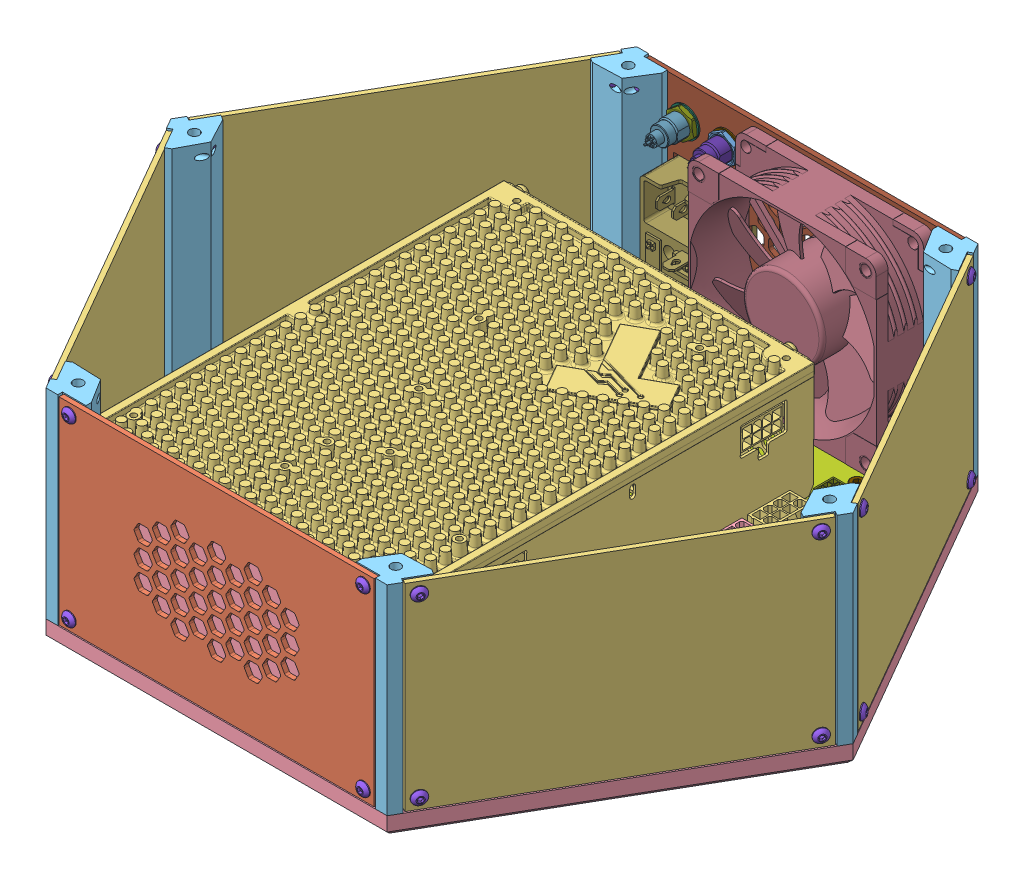
SolidWorks assembly base_assembly, configuration Default. Lengths in mm.
Overall size (362.5 93.4 376.72).
538 component instances, 72 part files, 51 mates.
Components (placement in the parent):
- psu_assembly-1: psu_assembly [Default] at (-81.5 8 97.5737) x (0 0 1) z (-1 0 0) size (187.35 61.91 139.14)
  - psu_mount-1: psu_mount [Default] at (-68 0 0) x (0 0 -1) z (1 0 0) size (39 54 68)
  - socket head cap screw_am-1: socket head cap screw_am [B18.3.1M - 3 x 0.5 x 8 Hex SHCS -- 8NHX] at (-64.25 14 3) x (0 0 -1) z (-0.998649 -0.051963 0) size (11 5.5 5.5)
  - socket head cap screw_am-2: socket head cap screw_am [B18.3.1M - 3 x 0.5 x 8 Hex SHCS -- 8NHX] at (-3.75 14 3) x (0 0 -1) z (-0.999942 -0.010799 0) size (11 5.5 5.5)
  - socket head cap screw_am-3: socket head cap screw_am [B18.3.1M - 3 x 0.5 x 8 Hex SHCS -- 8NHX] at (-3.75 50 3) x (0 0 -1) z (-0.998649 -0.051963 0) size (11 5.5 5.5)
  - IPC-5-1: IPC-5 [Default] at (-43.0401 19.0478 -84.9759) x (1 0 0) z (0 0.008727 0.999962) size (187.35 57.37 132.1)
- frame_bottom_assembly-1: frame_bottom_assembly [Default] at origin size (362.5 93.4 376.72)
  - bottom_plate_detail-1: bottom_plate_detail [Default] at (0 8 0) x (-0.5 0 -0.866025) z (-0.866025 0 0.5) size (290 8 251.15)
  - frame_pillar-1: frame_pillar [Default] at (72.5 8 -125.5737) x (-1 0 0) z (0 0 -1) size (20.77 85 15.16)
  - frame_pillar-3: frame_pillar [Default] at (-72.5 8 -125.5737) x (-0.5 0 0.866025) z (-0.866025 0 -0.5) size (20.77 85 15.16)
  - frame_pillar-4: frame_pillar [Default] at (-145 8 0) x (0.5 0 0.866025) z (-0.866025 0 0.5) size (20.77 85 15.16)
  - frame_pillar-5: frame_pillar [Default] at (-72.5 8 125.5737) size (20.77 85 15.16)
  - frame_pillar-6: frame_pillar [Default] at (72.5 8 125.5737) x (0.5 0 -0.866025) z (0.866025 0 0.5) size (20.77 85 15.16)
  - frame_pillar-7: frame_pillar [Default] at (145 8 0) x (-0.5 0 -0.866025) z (0.866025 0 -0.5) size (20.77 85 15.16)
  - socket countersunk head screw_am-5: socket countersunk head screw_am [B18.3.5M - 5 x 0.8 x 12 Socket FCHS  -- 12N] at (-70 0 38.5737) x (0 1 0) z (0 0 1) size (12 9.75 9.75)
  - socket countersunk head screw_am-6: socket countersunk head screw_am [B18.3.5M - 5 x 0.8 x 12 Socket FCHS  -- 12N] at (-50 0 38.5737) x (0 1 0) z (-0.110565 0 -0.993869) size (12 9.75 9.75)
  - socket countersunk head screw_am-7: socket countersunk head screw_am [B18.3.5M - 5 x 0.8 x 12 Socket FCHS  -- 12N] at (-50 0 88.5737) x (0 1 0) z (0 0 1) size (12 9.75 9.75)
  - socket countersunk head screw_am-8: socket countersunk head screw_am [B18.3.5M - 5 x 0.8 x 12 Socket FCHS  -- 12N] at (-70 0 88.5737) x (0 1 0) z (0 0 1) size (12 9.75 9.75)
  - socket countersunk head screw_am-9: socket countersunk head screw_am [B18.3.5M - 5 x 0.8 x 16 Socket FCHS  -- 16N] at (67.5 -0.4 116.9134) x (0 1 0) z (0 0 1) size (16 9.75 9.75)
  - socket countersunk head screw_am-10: socket countersunk head screw_am [B18.3.5M - 5 x 0.8 x 16 Socket FCHS  -- 16N] at (-67.5 -0.4 116.9134) x (0 1 0) z (0 0 1) size (16 9.75 9.75)
  - socket countersunk head screw_am-11: socket countersunk head screw_am [B18.3.5M - 5 x 0.8 x 16 Socket FCHS  -- 16N] at (-135 -0.4 0) x (0 1 0) z (0 0 1) size (16 9.75 9.75)
  - socket countersunk head screw_am-12: socket countersunk head screw_am [B18.3.5M - 5 x 0.8 x 16 Socket FCHS  -- 16N] at (-67.5 -0.4 -116.9134) x (0 1 0) z (0 0 1) size (16 9.75 9.75)
  - socket countersunk head screw_am-13: socket countersunk head screw_am [B18.3.5M - 5 x 0.8 x 16 Socket FCHS  -- 16N] at (67.5 -0.4 -116.9134) x (0 1 0) z (0 0 1) size (16 9.75 9.75)
  - socket countersunk head screw_am-14: socket countersunk head screw_am [B18.3.5M - 5 x 0.8 x 16 Socket FCHS  -- 16N] at (135 -0.4 0) x (0 1 0) z (0 0 1) size (16 9.75 9.75)
  - bottom_plate_cover-1: bottom_plate_cover [Default] at (124.7077 7 -108) x (-1 0 0) z (0 0 -1) size (247.87 1 216)
  - socket button head cap screw_am-1: socket button head cap screw_am [B18.3.4M - 3 x 0.5 x 6 SBHCS --N] at (120 9.65 0) x (0 -1 0) z (0 0 1) size (7.65 5.7 5.7) (hidden)
  - socket button head cap screw_am-2: socket button head cap screw_am [B18.3.4M - 3 x 0.5 x 6 SBHCS --N] at (60 9.65 103.923) x (0 -1 0) z (0 0 1) size (7.65 5.7 5.7) (hidden)
  - socket button head cap screw_am-3: socket button head cap screw_am [B18.3.4M - 3 x 0.5 x 6 SBHCS --N] at (-120 9.65 0) x (0 -1 0) z (0 0 1) size (7.65 5.7 5.7)
  - socket button head cap screw_am-4: socket button head cap screw_am [B18.3.4M - 3 x 0.5 x 6 SBHCS --N] at (-60 9.65 -103.923) x (0 -1 0) z (0 0 1) size (7.65 5.7 5.7)
  - socket button head cap screw_am-5: socket button head cap screw_am [B18.3.4M - 3 x 0.5 x 6 SBHCS --N] at (60 9.65 -103.923) x (0 -1 0) z (0 0 1) size (7.65 5.7 5.7)
  - nutsert_M3-4: nutsert_M3 [Default] at (60 5.5 -86.077) x (0.927804 0 -0.373067) z (0.373067 0 0.927804) size (5.3 2.75 5.3)
  - M3_standoff-1: M3_standoff [Default] at (60 8 -86.077) size (6.35 11 5.5)
  - M3_standoff-2: M3_standoff [Default] at (120 8 0) x (0.382257 0 -0.924056) z (0.924056 0 0.382257) size (6.35 11 5.5)
  - M3_standoff-3: M3_standoff [Default] at (60 8 103.923) size (6.35 11 5.5)
  - nutsert_M3-5: nutsert_M3 [Default] at (-90 5.5 -6.43) x (0.927804 0 -0.373067) z (0.373067 0 0.927804) size (5.3 2.75 5.3)
  - nutsert_M3-6: nutsert_M3 [Default] at (-110 5.5 13.57) x (0.927804 0 -0.373067) z (0.373067 0 0.927804) size (5.3 2.75 5.3)
  - nutsert_M3-7: nutsert_M3 [Default] at (-90 5.5 13.57) x (0.927804 0 -0.373067) z (0.373067 0 0.927804) size (5.3 2.75 5.3)
  - nutsert_M3-8: nutsert_M3 [Default] at (-90 5.5 33.57) x (0.927804 0 -0.373067) z (0.373067 0 0.927804) size (5.3 2.75 5.3)
  - nutsert_M3-9: nutsert_M3 [Default] at (-90 5.5 -26.43) x (0.927804 0 -0.373067) z (0.373067 0 0.927804) size (5.3 2.75 5.3)
- electronics_panel-1: electronics_panel [Default] at (-22.8265 182.5758 -40.206) x (-1 0 0) z (0 -1 0) size (134 36.39 84)
  - side_cover_fan-1: side_cover_fan [Default] at (-89.8265 83.3677 174.0758) size (134 2 84)
  - IEC 320 Switched-1: IEC 320 Switched [Default] at (4.4235 85.3677 118.9258) x (0 0 1) z (-1 0 0) size (58.1 34.87 32.67)
  - Noctua nf-a8-pwm fan 80x80x25-1: Noctua nf-a8-pwm fan 80x80x25 [По умолчанию] at (-39.0776 83.4677 131.8269) x (1 0 0.00003) z (0 -1 0) size (80 80 27.24)
  - socket button head cap screw_am-1: socket button head cap screw_am [B18.3.4M - 4 x 0.7 x 4 SBHCS --N] at (-74.5765 87.5677 96.3258) x (0 -1 0) z (0 0 1) size (6.2 7.6 7.6)
  - socket button head cap screw_am-2: socket button head cap screw_am [B18.3.4M - 4 x 0.7 x 4 SBHCS --N] at (-3.0765 87.5677 96.3258) x (0 -1 0) z (0 0 1) size (6.2 7.6 7.6)
  - socket button head cap screw_am-3: socket button head cap screw_am [B18.3.4M - 4 x 0.7 x 4 SBHCS --N] at (-3.0765 87.5677 167.8258) x (0 -1 0) z (0 0 1) size (6.2 7.6 7.6)
  - socket button head cap screw_am-4: socket button head cap screw_am [B18.3.4M - 4 x 0.7 x 4 SBHCS --N] at (-74.5765 87.5677 167.8258) x (0 -1 0) z (0 0 1) size (6.2 7.6 7.6)
  - egg_0b_307_cll-1: egg_0b_307_cll [Default] at (26.9235 88.8686 104.5758) x (-1 0 0) z (0 -1 0) size (12.77 13.42 20.7)
    - egg_0b_307_cll_1-1: egg_0b_307_cll_1 [Default] at (0 0 2.3009) size (10 10 20.7)
    - egg_0b_307_cll_2-1: egg_0b_307_cll_2 [Default] at (0 0 -1.0491) size (12.5 12.5 1.36)
    - egg_0b_307_cll_3-1: egg_0b_307_cll_3 [Default] at (0 0 -1.2991) size (12.77 13.42 2.93)
  - egg_0b_309_cll-1: egg_0b_309_cll [Default] at (8.9235 86.5677 104.5758) x (1 0 0) z (0 -1 0) size (12.5 12.5 20.23)
    - egg_0b_309_cll_1-1: egg_0b_309_cll_1 [Default] at origin size (10 10 20.23)
    - egg_0b_309_cll_2-1: egg_0b_309_cll_2 [Default] at (0 0 -4.6) size (12.5 12.5 1.3)
    - egg_0b_309_cll_3-1: egg_0b_309_cll_3 [Default] at (0 0 -4.85) size (11 12.4 2.02)
- socket button head cap screw_am-2: socket button head cap screw_am [B18.3.4M - 3 x 0.5 x 10 SBHCS --N] at (78.9289 13 -117.7384) x (-0.866025 0 0.5) z (-0.480675 0.27533 -0.832553) size (11.65 5.7 5.7)
- socket button head cap screw_am-3: socket button head cap screw_am [B18.3.4M - 3 x 0.5 x 10 SBHCS --N] at (141.4289 13 -9.4853) x (-0.866025 0 0.5) z (-0.480675 0.27533 -0.832553) size (11.65 5.7 5.7)
- socket button head cap screw_am-4: socket button head cap screw_am [B18.3.4M - 3 x 0.5 x 10 SBHCS --N] at (141.4289 88 -9.4853) x (-0.866025 0 0.5) z (-0.20533 0.911789 -0.355642) size (11.65 5.7 5.7)
- socket button head cap screw_am-5: socket button head cap screw_am [B18.3.4M - 3 x 0.5 x 10 SBHCS --N] at (78.9289 88 -117.7384) x (-0.866025 0 0.5) z (-0.480675 0.27533 -0.832553) size (11.65 5.7 5.7)
- socket button head cap screw_am-23: socket button head cap screw_am [B18.3.4M - 3 x 0.5 x 10 SBHCS --N] at (62.5 88 -127.2237) x (0 0 1) z (-0.900742 0.434355 0) size (11.65 5.7 5.7)
- socket button head cap screw_am-24: socket button head cap screw_am [B18.3.4M - 3 x 0.5 x 10 SBHCS --N] at (-62.5 88 -127.2237) x (0 0 1) z (-0.900742 0.434355 0) size (11.65 5.7 5.7)
- socket button head cap screw_am-25: socket button head cap screw_am [B18.3.4M - 3 x 0.5 x 10 SBHCS --N] at (-62.5 13 -127.2237) x (0 0 1) z (-0.900742 0.434355 0) size (11.65 5.7 5.7)
- socket button head cap screw_am-26: socket button head cap screw_am [B18.3.4M - 3 x 0.5 x 10 SBHCS --N] at (62.5 13 -127.2237) x (0 0 1) z (-0.900742 0.434355 0) size (11.65 5.7 5.7)
- side_cover_vent-1: side_cover_vent [Default] at (-67 8.5 123.5737) x (1 0 0) z (0 -1 0) size (134 2 84)
- side_cover_full-1: side_cover_full [Default] at (73.5179 92.5 -119.8105) x (0.5 0 0.866025) z (0 1 0) size (134 2 84)
- socket button head cap screw_am-27: socket button head cap screw_am [B18.3.4M - 3 x 0.5 x 10 SBHCS --N] at (-62.5 88 127.2237) x (0 0 -1) z (0.743296 -0.668962 0) size (11.65 5.7 5.7)
- socket button head cap screw_am-28: socket button head cap screw_am [B18.3.4M - 3 x 0.5 x 10 SBHCS --N] at (62.5 88 127.2237) x (0 0 -1) z (0.743296 -0.668962 0) size (11.65 5.7 5.7)
- socket button head cap screw_am-29: socket button head cap screw_am [B18.3.4M - 3 x 0.5 x 10 SBHCS --N] at (62.5 13 127.2237) x (0 0 -1) z (0.743296 -0.668962 0) size (11.65 5.7 5.7)
- socket button head cap screw_am-30: socket button head cap screw_am [B18.3.4M - 3 x 0.5 x 10 SBHCS --N] at (-62.5 13 127.2237) x (0 0 -1) z (0.743296 -0.668962 0) size (11.65 5.7 5.7)
- demci_filter_0887-1: demci_filter_0887 [Default] at (0 50.5 122.3737) x (1 0 0) z (0 -1 0) size (97 2.4 71)
- socket button head cap screw_am-31: socket button head cap screw_am [B18.3.4M - 3 x 0.5 x 10 SBHCS --N] at (-78.9289 13 -117.7384) x (0.866025 0 0.5) z (-0.480675 0.27533 0.832553) size (11.65 5.7 5.7)
- socket button head cap screw_am-32: socket button head cap screw_am [B18.3.4M - 3 x 0.5 x 10 SBHCS --N] at (-141.4289 13 9.4853) x (0.866025 0 -0.5) z (0.480675 0.27533 0.832553) size (11.65 5.7 5.7)
- socket button head cap screw_am-33: socket button head cap screw_am [B18.3.4M - 3 x 0.5 x 10 SBHCS --N] at (78.9289 13 117.7384) x (-0.866025 0 -0.5) z (0.480675 0.27533 -0.832553) size (11.65 5.7 5.7)
- socket button head cap screw_am-34: socket button head cap screw_am [B18.3.4M - 3 x 0.5 x 10 SBHCS --N] at (-141.4289 13 -9.4853) x (0.866025 0 0.5) z (-0.480675 0.27533 0.832553) size (11.65 5.7 5.7)
- socket button head cap screw_am-35: socket button head cap screw_am [B18.3.4M - 3 x 0.5 x 10 SBHCS --N] at (-78.9289 13 117.7384) x (0.866025 0 -0.5) z (0.480675 0.27533 0.832553) size (11.65 5.7 5.7)
- socket button head cap screw_am-36: socket button head cap screw_am [B18.3.4M - 3 x 0.5 x 10 SBHCS --N] at (141.4289 13 9.4853) x (-0.866025 0 -0.5) z (0.480675 0.27533 -0.832553) size (11.65 5.7 5.7)
- socket button head cap screw_am-37: socket button head cap screw_am [B18.3.4M - 3 x 0.5 x 10 SBHCS --N] at (-141.4289 88 -9.4853) x (0.866025 0 0.5) z (-0.480675 0.27533 0.832553) size (11.65 5.7 5.7)
- socket button head cap screw_am-38: socket button head cap screw_am [B18.3.4M - 3 x 0.5 x 10 SBHCS --N] at (-78.9289 88 117.7384) x (0.866025 0 -0.5) z (0.480675 0.27533 0.832553) size (11.65 5.7 5.7)
- socket button head cap screw_am-39: socket button head cap screw_am [B18.3.4M - 3 x 0.5 x 10 SBHCS --N] at (141.4289 88 9.4853) x (-0.866025 0 -0.5) z (0.480675 0.27533 -0.832553) size (11.65 5.7 5.7)
- socket button head cap screw_am-40: socket button head cap screw_am [B18.3.4M - 3 x 0.5 x 10 SBHCS --N] at (-78.9289 88 -117.7384) x (0.866025 0 0.5) z (-0.20533 0.911789 0.355642) size (11.65 5.7 5.7)
- socket button head cap screw_am-41: socket button head cap screw_am [B18.3.4M - 3 x 0.5 x 10 SBHCS --N] at (-141.4289 88 9.4853) x (0.866025 0 -0.5) z (0.20533 0.911789 0.355642) size (11.65 5.7 5.7)
- socket button head cap screw_am-42: socket button head cap screw_am [B18.3.4M - 3 x 0.5 x 10 SBHCS --N] at (78.9289 88 117.7384) x (-0.866025 0 -0.5) z (0.20533 0.911789 -0.355642) size (11.65 5.7 5.7)
- side_cover_full-10: side_cover_full [Default] at (-140.5179 92.5 -3.7631) x (0.5 0 -0.866025) z (0 1 0) size (134 2 84)
- side_cover_full-11: side_cover_full [Default] at (-73.5179 92.5 119.8105) x (-0.5 0 -0.866025) z (0 1 0) size (134 2 84)
- side_cover_full-12: side_cover_full [Default] at (140.5179 92.5 3.7631) x (-0.5 0 0.866025) z (0 1 0) size (134 2 84)
- zaphod-controller-1: zaphod-controller [Default] at (56 14 107.9) x (0 0 -1) z (0 1 0) size (199.92 69.34 18.57)
  - PKMCS0909E4000-1: PKMCS0909E4000 [Default] at (113.5 -47 -0.05) x (-1 0 0) z (0 -1 0) size (9 1.9 9)
    - COMPOUND-1: COMPOUND [Default] at origin size (9 1.9 9)
  - MOLEX_47053-1000-1: MOLEX_47053-1000 [Default] at (166.5524 -41.075 4.15) x (0.866025 0.5 0) z (0.5 -0.866025 0) size (10.2 13.5 5.84)
    - SOLID-1: SOLID [Default] at origin size (10.2 13.5 5.84)
  - SOIC127P1032X265-16L87-1: SOIC127P1032X265-16L87 [Default] at (151.3126 -39.0334 1.65) x (0.5 -0.866025 0) z (0 0 1) size (10.08 10.17 2)
    - COMPOUND_2-1: COMPOUND_2 [Default] at origin size (10.08 10.17 2)
  - CAPC1608X90-1: CAPC1608X90 [Default] at (147.0091 -44.05 -0.05) x (0 -1 0) z (0 0 -1) size (1.6 0.8 0.9)
    - COMPOUND_3-1: COMPOUND_3 [Default] at origin size (1.6 0.8 0.9)
  - CAPC1608X90-2: CAPC1608X90 [Default] at (147.1 -51.575 -0.05) x (0 -1 0) z (0 0 -1) size (1.6 0.8 0.9)
    - COMPOUND_3-1: COMPOUND_3 [Default] at origin size (1.6 0.8 0.9)
  - CAPC1608X90-3: CAPC1608X90 [Default] at (134.6 -51.575 -0.05) x (0 -1 0) z (0 0 -1) size (1.6 0.8 0.9)
    - COMPOUND_3-1: COMPOUND_3 [Default] at origin size (1.6 0.8 0.9)
  - CAPC1608X90-4: CAPC1608X90 [Default] at (134.6 -45.075 -0.05) x (0 -1 0) z (0 0 -1) size (1.6 0.8 0.9)
    - COMPOUND_3-1: COMPOUND_3 [Default] at origin size (1.6 0.8 0.9)
  - CAPC1608X90-5: CAPC1608X90 [Default] at (145.2978 -44.8154 1.65) x (0.866025 0.5 0) z (0 0 1) size (1.6 0.8 0.9)
    - COMPOUND_3-1: COMPOUND_3 [Default] at origin size (1.6 0.8 0.9)
  - CAPC1608X90-6: CAPC1608X90 [Default] at (160.5774 -38.8805 1.65) x (-0.866025 -0.5 0) z (0 0 1) size (1.6 0.8 0.9)
    - COMPOUND_3-1: COMPOUND_3 [Default] at origin size (1.6 0.8 0.9)
  - CAPC3225X170-1: CAPC3225X170 [Default] at (153.35 -43.55 -0.05) x (0 -1 0) z (0 0 -1) size (3.2 2.5 1.7)
    - COMPOUND_4-1: COMPOUND_4 [Default] at origin size (3.2 2.5 1.7)
  - CAPC3225X170-2: CAPC3225X170 [Default] at (131.85 -44.325 -0.05) x (0 -1 0) z (0 0 -1) size (3.2 2.5 1.7)
    - COMPOUND_4-1: COMPOUND_4 [Default] at origin size (3.2 2.5 1.7)
  - RESC1608X50-1: RESC1608X50 [Default] at (157.1 -45.05 -0.05) x (1 0 0) z (0 0 -1) size (1.6 0.8 0.5)
    - COMPOUND_5-1: COMPOUND_5 [Default] at origin size (1.6 0.8 0.5)
  - RESC1608X50-2: RESC1608X50 [Default] at (156.5275 -31.8657 1.65) x (-0.866025 -0.5 0) z (0 0 1) size (1.6 0.8 0.5)
    - COMPOUND_5-1: COMPOUND_5 [Default] at origin size (1.6 0.8 0.5)
  - RESC1608X50-3: RESC1608X50 [Default] at (157.1 -43.3 -0.05) x (1 0 0) z (0 0 -1) size (1.6 0.8 0.5)
    - COMPOUND_5-1: COMPOUND_5 [Default] at origin size (1.6 0.8 0.5)
  - RESC1608X50-4: RESC1608X50 [Default] at (157.4525 -33.4678 1.65) x (-0.866025 -0.5 0) z (0 0 1) size (1.6 0.8 0.5)
    - COMPOUND_5-1: COMPOUND_5 [Default] at origin size (1.6 0.8 0.5)
  - SOP65P780X200-24L40-1: SOP65P780X200-24L40 [Default] at (140.85 -47.8 -0.25) x (1 0 0) z (0 1 0) size (7.9 2.02 8.63)
    - SOLID_2-1: SOLID_2 [Default] at origin size (7.9 2.02 8.63)
  - MOLEX_NANOFIT_1053101110-1: MOLEX_NANOFIT_1053101110 [Default] at (158.2 -24.35 6.5) x (-1 0 0) z (0 0 1) size (13.44 8.86 13.71)
    - SOLID_3-1: SOLID_3 [Default] at origin size (13.44 8.86 13.71)
  - SOT95P240X110-3L16-1: SOT95P240X110-3L16 [Default] at (179 -22.5 -0.05) x (0 1 0) z (0 0 -1) size (2.91 3.01 1.23)
    - COMPOUND_6-1: COMPOUND_6 [Default] at origin size (2.91 3.01 1.23)
  - RESC1608X50-5: RESC1608X50 [Default] at (182.7 -19.3 -0.05) x (-1 0 0) z (0 0 -1) size (1.6 0.8 0.5)
    - COMPOUND_5-1: COMPOUND_5 [Default] at origin size (1.6 0.8 0.5)
  - MOLEX_NANOFIT_1053091106-1: MOLEX_NANOFIT_1053091106 [Default] at (181.5175 -33.225 6.5) x (0.866025 0.5 0) z (0 0 1) size (15.94 6.34 13.71)
    - SOLID_4-1: SOLID_4 [Default] at origin size (15.94 6.34 13.71)
  - MOLEX_NANOFIT_1053101108-1: MOLEX_NANOFIT_1053101108 [Default] at (194.05 -16.05 6.55) x (0 1 0) z (0 0 1) size (10.94 8.84 13.71)
    - SOLID_5-1: SOLID_5 [Default] at origin size (10.94 8.84 13.71)
  - MOLEX_NANOFIT_1053101106-1: MOLEX_NANOFIT_1053101106 [Default] at (181 -6.25 6.5) x (-1 0 0) z (0 0 1) size (8.44 8.84 13.71)
    - SOLID_6-1: SOLID_6 [Default] at origin size (8.44 8.84 13.71)
  - 61300211121-1: 61300211121 [Default] at (133.83 -18.6 2.65) x (1 0 0) z (0 -1 0) size (5.08 11.54 2.54)
    - SOLID_7-1: SOLID_7 [Default] at origin size (0.64 11.54 0.64)
    - SOLID_8-1: SOLID_8 [Default] at origin size (0.64 11.54 0.64)
    - SOLID_9-1: SOLID_9 [Default] at origin size (5.08 2.54 2.54)
  - RESC1608X50-6: RESC1608X50 [Default] at (132.8 -34.6 1.65) x (-1 0 0) z (0 0 1) size (1.6 0.8 0.5)
    - COMPOUND_5-1: COMPOUND_5 [Default] at origin size (1.6 0.8 0.5)
  - RESC1608X50-7: RESC1608X50 [Default] at (133.8 -21.4 1.65) x (-1 0 0) z (0 0 1) size (1.6 0.8 0.5)
    - COMPOUND_5-1: COMPOUND_5 [Default] at origin size (1.6 0.8 0.5)
  - RESC1608X50-8: RESC1608X50 [Default] at (57.7 -27.2 -0.05) x (1 0 0) z (0 0 -1) size (1.6 0.8 0.5)
    - COMPOUND_5-1: COMPOUND_5 [Default] at origin size (1.6 0.8 0.5)
  - MOLEX_SABRE_431600102-1: MOLEX_SABRE_431600102 [Default] at (15.5 -11.45 9.05) x (0 1 0) z (1 0 0) size (21.08 18.57 13.39)
    - SOLID_10-1: SOLID_10 [Default] at origin size (21.08 18.57 13.39)
  - MOLEX_MICROFITJR_039281083-1: MOLEX_MICROFITJR_039281083 [Default] at (53.3 -7.5 1.65) x (-1 0 0) z (0 1 0) size (18.8 16.3 11)
    - SOLID_11-1: SOLID_11 [Default] at origin size (18.8 16.3 11)
  - MOLEX_MICROFITJR_039281083-2: MOLEX_MICROFITJR_039281083 [Default] at (88.3 -7.5 1.65) x (-1 0 0) z (0 1 0) size (18.8 16.3 11)
    - SOLID_11-1: SOLID_11 [Default] at origin size (18.8 16.3 11)
  - MOLEX_MICROFITJR_039281083-3: MOLEX_MICROFITJR_039281083 [Default] at (123.3 -7.5 1.65) x (-1 0 0) z (0 1 0) size (18.8 16.3 11)
    - SOLID_11-1: SOLID_11 [Default] at origin size (18.8 16.3 11)
  - MOLEX_MICROFITJR_039281083-4: MOLEX_MICROFITJR_039281083 [Default] at (158.3 -7.5 1.65) x (-1 0 0) z (0 1 0) size (18.8 16.3 11)
    - SOLID_11-1: SOLID_11 [Default] at origin size (18.8 16.3 11)
  - MOLEX_MICROFITJR_039281043-1: MOLEX_MICROFITJR_039281043 [Default] at (37.1 -7.5 1.65) x (-1 0 0) z (0 1 0) size (10.4 16.3 11)
    - SOLID_12-1: SOLID_12 [Default] at origin size (10.4 16.3 11)
  - MOLEX_MICROFITJR_039281043-2: MOLEX_MICROFITJR_039281043 [Default] at (72.1 -7.5 1.65) x (-1 0 0) z (0 1 0) size (10.4 16.3 11)
    - SOLID_12-1: SOLID_12 [Default] at origin size (10.4 16.3 11)
  - MOLEX_MICROFITJR_039281043-3: MOLEX_MICROFITJR_039281043 [Default] at (107.1 -7.5 1.65) x (-1 0 0) z (0 1 0) size (10.4 16.3 11)
    - SOLID_12-1: SOLID_12 [Default] at origin size (10.4 16.3 11)
  - MOLEX_MICROFITJR_039281043-4: MOLEX_MICROFITJR_039281043 [Default] at (142.1 -7.5 1.65) x (-1 0 0) z (0 1 0) size (10.4 16.3 11)
    - SOLID_12-1: SOLID_12 [Default] at origin size (10.4 16.3 11)
  - PULSE_PA2050-1: PULSE_PA2050 [Default] at (84.85 -28.9 1.65) x (0 -1 0) z (-1 0 0) size (22.23 12.2 19.25)
    - SOLID_13-1: SOLID_13 [Default] at origin size (22.23 12.2 19.25)
  - 61300611121-1: 61300611121 [Default] at (117.35 -57.1 2.65) x (1 0 0) z (0 -1 0) size (15.24 11.54 2.54)
    - SOLID_14-1: SOLID_14 [Default] at origin size (0.64 11.54 0.64)
    - SOLID_15-1: SOLID_15 [Default] at origin size (0.64 11.54 0.64)
    - SOLID_16-1: SOLID_16 [Default] at origin size (0.64 11.54 0.64)
    - SOLID_17-1: SOLID_17 [Default] at origin size (0.64 11.54 0.64)
    - SOLID_18-1: SOLID_18 [Default] at origin size (0.64 11.54 0.64)
    - SOLID_19-1: SOLID_19 [Default] at origin size (0.64 11.54 0.64)
    - SOLID_20-1: SOLID_20 [Default] at origin size (15.24 2.54 2.54)
  - LEDC1608X80L40-1: LEDC1608X80L40 [Default] at (141.8 -55.6 1.75) x (-0.5 0.866025 0) z (0.866025 0.5 0) size (1.61 0.75 0.81)
    - COMPOUND_7-1: COMPOUND_7 [Default] at origin size (1.61 0.75 0.81)
  - LEDC1608X80L40-2: LEDC1608X80L40 [Default] at (139.2 -57 1.75) x (-0.5 0.866025 0) z (0.866025 0.5 0) size (1.61 0.75 0.81)
    - COMPOUND_7-1: COMPOUND_7 [Default] at origin size (1.61 0.75 0.81)
  - LEDC1608X80L40-3: LEDC1608X80L40 [Default] at (144.2 -54.3 1.75) x (-0.5 0.866025 0) z (0.866025 0.5 0) size (1.61 0.75 0.81)
    - COMPOUND_7-1: COMPOUND_7 [Default] at origin size (1.61 0.75 0.81)
  - SOT95P240X110-3L16-2: SOT95P240X110-3L16 [Default] at (54.05 -21.3 1.65) x (0 -1 0) z (0 0 1) size (2.91 3.01 1.23)
    - COMPOUND_6-1: COMPOUND_6 [Default] at origin size (2.91 3.01 1.23)
  - CAPC1608X90-7: CAPC1608X90 [Default] at (169.2907 -8.1731 -0.05) x (-1 0 0) z (0 0 -1) size (1.6 0.8 0.9)
    - COMPOUND_3-1: COMPOUND_3 [Default] at origin size (1.6 0.8 0.9)
  - CAPC3225X170-3: CAPC3225X170 [Default] at (95.5 -47.25 1.65) size (3.2 2.5 1.7)
    - COMPOUND_4-1: COMPOUND_4 [Default] at origin size (3.2 2.5 1.7)
  - CAPC4532X180-1: CAPC4532X180 [Default] at (59.2 -44 1.65) size (4.5 3.2 1.8)
    - COMPOUND_8-1: COMPOUND_8 [Default] at origin size (4.5 3.2 1.8)
  - CAPC4532X180-2: CAPC4532X180 [Default] at (59.2 -39.5 1.65) size (4.5 3.2 1.8)
    - COMPOUND_8-1: COMPOUND_8 [Default] at origin size (4.5 3.2 1.8)
  - CAPC1608X90-8: CAPC1608X90 [Default] at (96.275 -44.5 1.65) x (-1 0 0) z (0 0 1) size (1.6 0.8 0.9)
    - COMPOUND_3-1: COMPOUND_3 [Default] at origin size (1.6 0.8 0.9)
  - CAPC4532X180-3: CAPC4532X180 [Default] at (59.2 -35 1.65) size (4.5 3.2 1.8)
    - COMPOUND_8-1: COMPOUND_8 [Default] at origin size (4.5 3.2 1.8)
  - CAPC4532X180-4: CAPC4532X180 [Default] at (59.2 -30.5 1.65) size (4.5 3.2 1.8)
    - COMPOUND_8-1: COMPOUND_8 [Default] at origin size (4.5 3.2 1.8)
  - CAPC1608X90-9: CAPC1608X90 [Default] at (32.7 -25.25 1.65) x (-1 0 0) z (0 0 1) size (1.6 0.8 0.9)
    - COMPOUND_3-1: COMPOUND_3 [Default] at origin size (1.6 0.8 0.9)
  - CAPC1608X90-10: CAPC1608X90 [Default] at (105.725 -45 1.65) x (-1 0 0) z (0 0 1) size (1.6 0.8 0.9)
    - COMPOUND_3-1: COMPOUND_3 [Default] at origin size (1.6 0.8 0.9)
  - CAPC1608X90-11: CAPC1608X90 [Default] at (29.2 -16.25 1.65) size (1.6 0.8 0.9)
    - COMPOUND_3-1: COMPOUND_3 [Default] at origin size (1.6 0.8 0.9)
  - CAPC1608X90-12: CAPC1608X90 [Default] at (29.45 -27 1.65) size (1.6 0.8 0.9)
    - COMPOUND_3-1: COMPOUND_3 [Default] at origin size (1.6 0.8 0.9)
  - CAPC1608X90-13: CAPC1608X90 [Default] at (104.75 -51 1.65) x (0 1 0) z (0 0 1) size (1.6 0.8 0.9)
    - COMPOUND_3-1: COMPOUND_3 [Default] at origin size (1.6 0.8 0.9)
  - CAPC3225X170-4: CAPC3225X170 [Default] at (103 -56 1.65) x (0 -1 0) z (0 0 1) size (3.2 2.5 1.7)
    - COMPOUND_4-1: COMPOUND_4 [Default] at origin size (3.2 2.5 1.7)
  - CAPC1608X90-14: CAPC1608X90 [Default] at (29.2 -24 1.65) x (-1 0 0) z (0 0 1) size (1.6 0.8 0.9)
    - COMPOUND_3-1: COMPOUND_3 [Default] at origin size (1.6 0.8 0.9)
  - CAPC3225X170-5: CAPC3225X170 [Default] at (106.5 -56 1.65) x (0 -1 0) z (0 0 1) size (3.2 2.5 1.7)
    - COMPOUND_4-1: COMPOUND_4 [Default] at origin size (3.2 2.5 1.7)
  - CAPC1608X90-15: CAPC1608X90 [Default] at (29.2 -22.25 1.65) x (-1 0 0) z (0 0 1) size (1.6 0.8 0.9)
    - COMPOUND_3-1: COMPOUND_3 [Default] at origin size (1.6 0.8 0.9)
  - CAPC2012X110-1: CAPC2012X110 [Default] at (41.1 -25.3 -0.05) x (1 0 0) z (0 0 -1) size (2 1.2 1.1)
    - COMPOUND_9-1: COMPOUND_9 [Default] at origin size (2 1.2 1.1)
  - CAPC2012X110-2: CAPC2012X110 [Default] at (49.8 -17.05 1.65) x (-1 0 0) z (0 0 1) size (2 1.2 1.1)
    - COMPOUND_9-1: COMPOUND_9 [Default] at origin size (2 1.2 1.1)
  - CAPC3225X170-6: CAPC3225X170 [Default] at (79.5 -47.25 1.65) size (3.2 2.5 1.7)
    - COMPOUND_4-1: COMPOUND_4 [Default] at origin size (3.2 2.5 1.7)
  - CAPC2012X110-3: CAPC2012X110 [Default] at (55.3 -17.05 1.65) x (0 -1 0) z (0 0 1) size (2 1.2 1.1)
    - COMPOUND_9-1: COMPOUND_9 [Default] at origin size (2 1.2 1.1)
  - CAPC1608X90-16: CAPC1608X90 [Default] at (80.275 -44.5 1.65) x (-1 0 0) z (0 0 1) size (1.6 0.8 0.9)
    - COMPOUND_3-1: COMPOUND_3 [Default] at origin size (1.6 0.8 0.9)
  - CAPC1608X90-17: CAPC1608X90 [Default] at (89.725 -45 1.65) x (-1 0 0) z (0 0 1) size (1.6 0.8 0.9)
    - COMPOUND_3-1: COMPOUND_3 [Default] at origin size (1.6 0.8 0.9)
  - CAPC1608X90-18: CAPC1608X90 [Default] at (88.75 -51 1.65) x (0 1 0) z (0 0 1) size (1.6 0.8 0.9)
    - COMPOUND_3-1: COMPOUND_3 [Default] at origin size (1.6 0.8 0.9)
  - CAPC3225X170-7: CAPC3225X170 [Default] at (90.5 -56 1.65) x (0 -1 0) z (0 0 1) size (3.2 2.5 1.7)
    - COMPOUND_4-1: COMPOUND_4 [Default] at origin size (3.2 2.5 1.7)
  - CAPC3225X170-8: CAPC3225X170 [Default] at (68.65 -51.8 1.65) x (-1 0 0) z (0 0 1) size (3.2 2.5 1.7)
    - COMPOUND_4-1: COMPOUND_4 [Default] at origin size (3.2 2.5 1.7)
  - CAPC3225X170-9: CAPC3225X170 [Default] at (87 -56 1.65) x (0 -1 0) z (0 0 1) size (3.2 2.5 1.7)
    - COMPOUND_4-1: COMPOUND_4 [Default] at origin size (3.2 2.5 1.7)
  - CAPC1608X90-19: CAPC1608X90 [Default] at (103.8 -20 1.65) x (-1 0 0) z (0 0 1) size (1.6 0.8 0.9)
    - COMPOUND_3-1: COMPOUND_3 [Default] at origin size (1.6 0.8 0.9)
  - CAPC1608X90-20: CAPC1608X90 [Default] at (128 -25.5 -0.05) x (0 1 0) z (0 0 -1) size (1.6 0.8 0.9)
    - COMPOUND_3-1: COMPOUND_3 [Default] at origin size (1.6 0.8 0.9)
  - CAPC1608X90-21: CAPC1608X90 [Default] at (100 -36.6 1.65) x (-1 0 0) z (0 0 1) size (1.6 0.8 0.9)
    - COMPOUND_3-1: COMPOUND_3 [Default] at origin size (1.6 0.8 0.9)
  - CAPC1608X90-22: CAPC1608X90 [Default] at (129.75 -25.5 -0.05) x (0 1 0) z (0 0 -1) size (1.6 0.8 0.9)
    - COMPOUND_3-1: COMPOUND_3 [Default] at origin size (1.6 0.8 0.9)
  - CAPC1608X90-23: CAPC1608X90 [Default] at (131.6 -55.1 1.65) x (0.866025 0.5 0) z (0 0 1) size (1.6 0.8 0.9)
    - COMPOUND_3-1: COMPOUND_3 [Default] at origin size (1.6 0.8 0.9)
  - CAPC1608X90-24: CAPC1608X90 [Default] at (146.5478 -46.9805 1.65) x (0.866025 0.5 0) z (0 0 1) size (1.6 0.8 0.9)
    - COMPOUND_3-1: COMPOUND_3 [Default] at origin size (1.6 0.8 0.9)
  - CAPC1608X90-25: CAPC1608X90 [Default] at (123.6 -34.9 -0.05) x (-1 0 0) z (0 0 -1) size (1.6 0.8 0.9)
    - COMPOUND_3-1: COMPOUND_3 [Default] at origin size (1.6 0.8 0.9)
  - CAPC1608X90-26: CAPC1608X90 [Default] at (123.6 -29.6 -0.05) x (1 0 0) z (0 0 -1) size (1.6 0.8 0.9)
    - COMPOUND_3-1: COMPOUND_3 [Default] at origin size (1.6 0.8 0.9)
  - CAPC1608X90-27: CAPC1608X90 [Default] at (118.5 -21.6 1.65) size (1.6 0.8 0.9)
    - COMPOUND_3-1: COMPOUND_3 [Default] at origin size (1.6 0.8 0.9)
  - CAPC1608X90-28: CAPC1608X90 [Default] at (103.8 -21.8 1.65) x (-1 0 0) z (0 0 1) size (1.6 0.8 0.9)
    - COMPOUND_3-1: COMPOUND_3 [Default] at origin size (1.6 0.8 0.9)
  - CAPC1608X90-29: CAPC1608X90 [Default] at (100 -38.6 1.65) x (-1 0 0) z (0 0 1) size (1.6 0.8 0.9)
    - COMPOUND_3-1: COMPOUND_3 [Default] at origin size (1.6 0.8 0.9)
  - CAPC1608X90-30: CAPC1608X90 [Default] at (124.5 -25.5 -0.05) x (0 1 0) z (0 0 -1) size (1.6 0.8 0.9)
    - COMPOUND_3-1: COMPOUND_3 [Default] at origin size (1.6 0.8 0.9)
  - CAPC1608X90-31: CAPC1608X90 [Default] at (118.2 -42.4 1.65) x (-1 0 0) z (0 0 1) size (1.6 0.8 0.9)
    - COMPOUND_3-1: COMPOUND_3 [Default] at origin size (1.6 0.8 0.9)
  - CAPC1608X90-32: CAPC1608X90 [Default] at (126.25 -25.5 -0.05) x (0 1 0) z (0 0 -1) size (1.6 0.8 0.9)
    - COMPOUND_3-1: COMPOUND_3 [Default] at origin size (1.6 0.8 0.9)
  - CAPC1608X90-33: CAPC1608X90 [Default] at (128.8 -36.6 1.65) size (1.6 0.8 0.9)
    - COMPOUND_3-1: COMPOUND_3 [Default] at origin size (1.6 0.8 0.9)
  - CAPC1608X90-34: CAPC1608X90 [Default] at (128.8 -34.6 1.65) size (1.6 0.8 0.9)
    - COMPOUND_3-1: COMPOUND_3 [Default] at origin size (1.6 0.8 0.9)
  - CAPC1608X90-35: CAPC1608X90 [Default] at (30 -11.009 -0.05) x (-1 0 0) z (0 0 -1) size (1.6 0.8 0.9)
    - COMPOUND_3-1: COMPOUND_3 [Default] at origin size (1.6 0.8 0.9)
  - CAPC1608X90-36: CAPC1608X90 [Default] at (64.9267 -11 -0.05) x (-1 0 0) z (0 0 -1) size (1.6 0.8 0.9)
    - COMPOUND_3-1: COMPOUND_3 [Default] at origin size (1.6 0.8 0.9)
  - CAPC1608X90-37: CAPC1608X90 [Default] at (100 -11 -0.05) x (-1 0 0) z (0 0 -1) size (1.6 0.8 0.9)
    - COMPOUND_3-1: COMPOUND_3 [Default] at origin size (1.6 0.8 0.9)
  - CAPC1608X90-38: CAPC1608X90 [Default] at (134.8 -11 -0.05) x (-1 0 0) z (0 0 -1) size (1.6 0.8 0.9)
    - COMPOUND_3-1: COMPOUND_3 [Default] at origin size (1.6 0.8 0.9)
  - CAPC1608X90-39: CAPC1608X90 [Default] at (90.298 -35.5 -0.05) x (-1 0 0) z (0 0 -1) size (1.6 0.8 0.9)
    - COMPOUND_3-1: COMPOUND_3 [Default] at origin size (1.6 0.8 0.9)
  - CAPC1608X90-40: CAPC1608X90 [Default] at (140.602 -20.7 -0.05) x (1 0 0) z (0 0 -1) size (1.6 0.8 0.9)
    - COMPOUND_3-1: COMPOUND_3 [Default] at origin size (1.6 0.8 0.9)
  - CAPC1608X90-41: CAPC1608X90 [Default] at (46.9727 -15.598 -0.05) x (0 -1 0) z (0 0 -1) size (1.6 0.8 0.9)
    - COMPOUND_3-1: COMPOUND_3 [Default] at origin size (1.6 0.8 0.9)
  - CAPC1608X90-42: CAPC1608X90 [Default] at (117 -15.598 -0.05) x (0 -1 0) z (0 0 -1) size (1.6 0.8 0.9)
    - COMPOUND_3-1: COMPOUND_3 [Default] at origin size (1.6 0.8 0.9)
  - CAPC1608X90-43: CAPC1608X90 [Default] at (81.9353 -15.5817 -0.05) x (0 -1 0) z (0 0 -1) size (1.6 0.8 0.9)
    - COMPOUND_3-1: COMPOUND_3 [Default] at origin size (1.6 0.8 0.9)
  - CAPC1608X90-44: CAPC1608X90 [Default] at (152 -15.6 -0.05) x (0 -1 0) z (0 0 -1) size (1.6 0.8 0.9)
    - COMPOUND_3-1: COMPOUND_3 [Default] at origin size (1.6 0.8 0.9)
  - CAPC1608X90-45: CAPC1608X90 [Default] at (187.9 -12.5 -0.05) x (1 0 0) z (0 0 -1) size (1.6 0.8 0.9)
    - COMPOUND_3-1: COMPOUND_3 [Default] at origin size (1.6 0.8 0.9)
  - CAPC1608X90-46: CAPC1608X90 [Default] at (187.9 -14.2 -0.05) x (1 0 0) z (0 0 -1) size (1.6 0.8 0.9)
    - COMPOUND_3-1: COMPOUND_3 [Default] at origin size (1.6 0.8 0.9)
  - CAPC1608X90-47: CAPC1608X90 [Default] at (187.9 -15.9 -0.05) x (1 0 0) z (0 0 -1) size (1.6 0.8 0.9)
    - COMPOUND_3-1: COMPOUND_3 [Default] at origin size (1.6 0.8 0.9)
  - CAPC1608X90-48: CAPC1608X90 [Default] at (187.9 -17.6 -0.05) x (1 0 0) z (0 0 -1) size (1.6 0.8 0.9)
    - COMPOUND_3-1: COMPOUND_3 [Default] at origin size (1.6 0.8 0.9)
  - CAPC1608X90-49: CAPC1608X90 [Default] at (187.9 -19.3 -0.05) x (1 0 0) z (0 0 -1) size (1.6 0.8 0.9)
    - COMPOUND_3-1: COMPOUND_3 [Default] at origin size (1.6 0.8 0.9)
  - CAPC1608X90-50: CAPC1608X90 [Default] at (159.3274 -36.7154 1.65) x (-0.866025 -0.5 0) z (0 0 1) size (1.6 0.8 0.9)
    - COMPOUND_3-1: COMPOUND_3 [Default] at origin size (1.6 0.8 0.9)
  - CAPC1608X90-51: CAPC1608X90 [Default] at (187.8692 -27.1 -0.05) x (1 0 0) z (0 0 -1) size (1.6 0.8 0.9)
    - COMPOUND_3-1: COMPOUND_3 [Default] at origin size (1.6 0.8 0.9)
  - CAPC1608X90-52: CAPC1608X90 [Default] at (187.8442 -25.4 -0.05) x (1 0 0) z (0 0 -1) size (1.6 0.8 0.9)
    - COMPOUND_3-1: COMPOUND_3 [Default] at origin size (1.6 0.8 0.9)
  - CAPC1608X90-53: CAPC1608X90 [Default] at (187.8692 -23.7 -0.05) x (1 0 0) z (0 0 -1) size (1.6 0.8 0.9)
    - COMPOUND_3-1: COMPOUND_3 [Default] at origin size (1.6 0.8 0.9)
  - CAPC1608X90-54: CAPC1608X90 [Default] at (187.9 -22 -0.05) x (1 0 0) z (0 0 -1) size (1.6 0.8 0.9)
    - COMPOUND_3-1: COMPOUND_3 [Default] at origin size (1.6 0.8 0.9)
  - CAPC1608X90-55: CAPC1608X90 [Default] at (132.775 -36.6 1.65) size (1.6 0.8 0.9)
    - COMPOUND_3-1: COMPOUND_3 [Default] at origin size (1.6 0.8 0.9)
  - CAPC1608X90-56: CAPC1608X90 [Default] at (57.7 -29.1 -0.05) x (-1 0 0) z (0 0 -1) size (1.6 0.8 0.9)
    - COMPOUND_3-1: COMPOUND_3 [Default] at origin size (1.6 0.8 0.9)
  - CAPC3225X170-10: CAPC3225X170 [Default] at (138.4 -31.6 1.65) size (3.2 2.5 1.7)
    - COMPOUND_4-1: COMPOUND_4 [Default] at origin size (3.2 2.5 1.7)
  - CAPC1608X90-57: CAPC1608X90 [Default] at (133.8 -23.1 1.65) size (1.6 0.8 0.9)
    - COMPOUND_3-1: COMPOUND_3 [Default] at origin size (1.6 0.8 0.9)
  - CAPC1608X90-58: CAPC1608X90 [Default] at (141.9 -32.375 1.65) x (0 1 0) z (0 0 1) size (1.6 0.8 0.9)
    - COMPOUND_3-1: COMPOUND_3 [Default] at origin size (1.6 0.8 0.9)
  - SOT95P240X110-3L16-3: SOT95P240X110-3L16 [Default] at (169.2907 -11.3731 -0.05) x (0 1 0) z (0 0 -1) size (2.91 3.01 1.23)
    - COMPOUND_6-1: COMPOUND_6 [Default] at origin size (2.91 3.01 1.23)
  - SOT95P240X110-3L16-4: SOT95P240X110-3L16 [Default] at (32.95 -15.25 1.65) x (-1 0 0) z (0 0 1) size (2.91 3.01 1.23)
    - COMPOUND_6-1: COMPOUND_6 [Default] at origin size (2.91 3.01 1.23)
  - SOT95P240X110-3L16-5: SOT95P240X110-3L16 [Default] at (42 -15.598 -0.05) x (0 1 0) z (0 0 -1) size (2.91 3.01 1.23)
    - COMPOUND_6-1: COMPOUND_6 [Default] at origin size (2.91 3.01 1.23)
  - SOT95P240X110-3L16-6: SOT95P240X110-3L16 [Default] at (112.2 -15.6 -0.05) x (0 1 0) z (0 0 -1) size (2.91 3.01 1.23)
    - COMPOUND_6-1: COMPOUND_6 [Default] at origin size (2.91 3.01 1.23)
  - SOT95P240X110-3L16-7: SOT95P240X110-3L16 [Default] at (77 -15.6 -0.05) x (0 1 0) z (0 0 -1) size (2.91 3.01 1.23)
    - COMPOUND_6-1: COMPOUND_6 [Default] at origin size (2.91 3.01 1.23)
  - SOT95P240X110-3L16-8: SOT95P240X110-3L16 [Default] at (147.2 -15.6 -0.05) x (0 1 0) z (0 0 -1) size (2.91 3.01 1.23)
    - COMPOUND_6-1: COMPOUND_6 [Default] at origin size (2.91 3.01 1.23)
  - DO-215AD-1: DO-215AD [Default] at (49.2 -15.598 -0.05) x (0 -1 0) z (0 0 -1) size (3.85 1.7 1.35)
    - COMPOUND_10-1: COMPOUND_10 [Default] at origin size (3.85 1.7 1.35)
  - DO-215AD-2: DO-215AD [Default] at (84.2 -15.6 -0.05) x (0 -1 0) z (0 0 -1) size (3.85 1.7 1.35)
    - COMPOUND_10-1: COMPOUND_10 [Default] at origin size (3.85 1.7 1.35)
  - DO-215AD-3: DO-215AD [Default] at (119.2 -15.598 -0.05) x (0 -1 0) z (0 0 -1) size (3.85 1.7 1.35)
    - COMPOUND_10-1: COMPOUND_10 [Default] at origin size (3.85 1.7 1.35)
  - DO-215AD-4: DO-215AD [Default] at (154.2 -15.6 -0.05) x (0 -1 0) z (0 0 -1) size (3.85 1.7 1.35)
    - COMPOUND_10-1: COMPOUND_10 [Default] at origin size (3.85 1.7 1.35)
  - SOT95P240X110-3L16-9: SOT95P240X110-3L16 [Default] at (179 -12.5 -0.05) x (0 1 0) z (0 0 -1) size (2.91 3.01 1.23)
    - COMPOUND_6-1: COMPOUND_6 [Default] at origin size (2.91 3.01 1.23)
  - SOT95P240X110-3L16-10: SOT95P240X110-3L16 [Default] at (175.1 -12.5 -0.05) x (0 1 0) z (0 0 -1) size (2.91 3.01 1.23)
    - COMPOUND_6-1: COMPOUND_6 [Default] at origin size (2.91 3.01 1.23)
  - SOT95P240X110-3L16-11: SOT95P240X110-3L16 [Default] at (175.1 -17.6 -0.05) x (0 -1 0) z (0 0 -1) size (2.91 3.01 1.23)
    - COMPOUND_6-1: COMPOUND_6 [Default] at origin size (2.91 3.01 1.23)
  - SOT95P240X110-3L16-12: SOT95P240X110-3L16 [Default] at (179 -17.6 -0.05) x (0 -1 0) z (0 0 -1) size (2.91 3.01 1.23)
    - COMPOUND_6-1: COMPOUND_6 [Default] at origin size (2.91 3.01 1.23)
  - SOT95P240X110-3L16-13: SOT95P240X110-3L16 [Default] at (171.2 -17.6 -0.05) x (0 -1 0) z (0 0 -1) size (2.91 3.01 1.23)
    - COMPOUND_6-1: COMPOUND_6 [Default] at origin size (2.91 3.01 1.23)
  - SOT95P240X110-3L16-14: SOT95P240X110-3L16 [Default] at (179 -27.8 -0.05) x (0 -1 0) z (0 0 -1) size (2.91 3.01 1.23)
    - COMPOUND_6-1: COMPOUND_6 [Default] at origin size (2.91 3.01 1.23)
  - SOT95P240X110-3L16-15: SOT95P240X110-3L16 [Default] at (175.1 -27.8 -0.05) x (0 -1 0) z (0 0 -1) size (2.91 3.01 1.23)
    - COMPOUND_6-1: COMPOUND_6 [Default] at origin size (2.91 3.01 1.23)
  - SOT95P240X110-3L16-16: SOT95P240X110-3L16 [Default] at (175.1 -22.5 -0.05) x (0 1 0) z (0 0 -1) size (2.91 3.01 1.23)
    - COMPOUND_6-1: COMPOUND_6 [Default] at origin size (2.91 3.01 1.23)
  - SOT95P240X110-3L16-17: SOT95P240X110-3L16 [Default] at (141.5 -27.4 1.65) x (0 -1 0) z (0 0 1) size (2.91 3.01 1.23)
    - COMPOUND_6-1: COMPOUND_6 [Default] at origin size (2.91 3.01 1.23)
  - 3225M_POLYFUSE-1: 3225M_POLYFUSE [Default] at (145.4685 -31.6 1.65) x (-1 0 0) z (0 1 0) size (3.22 0.68 2.58)
    - COMPOUND_11-1: COMPOUND_11 [Default] at origin size (3.22 0.68 2.58)
  - INDM7300x7300x355-1: INDM7300x7300x355 [Default] at (97 -54 2.65) x (-1 0 0) z (0 1 0) size (7.3 4.01 7.3)
    - COMPOUND_12-1: COMPOUND_12 [Default] at origin size (7.3 4.01 7.3)
  - INDM7300x7300x355-2: INDM7300x7300x355 [Default] at (81 -54 2.65) x (-1 0 0) z (0 1 0) size (7.3 4.01 7.3)
    - COMPOUND_12-1: COMPOUND_12 [Default] at origin size (7.3 4.01 7.3)
  - SON127P490X575X90-9T313X381-1: SON127P490X575X90-9T313X381 [Default] at (60.4 -22.55 1.7) x (0 -1 0) z (0 0 1) size (6.01 4.9 0.95)
    - SOLID_21-1: SOLID_21 [Default] at origin size (6.01 4.9 0.95)
  - SON127P490X575X90-9T313X381-2: SON127P490X575X90-9T313X381 [Default] at (68.65 -20.3 1.7) x (0 1 0) z (0 0 1) size (6.01 4.9 0.95)
    - SOLID_21-1: SOLID_21 [Default] at origin size (6.01 4.9 0.95)
  - SOT95P240X110-3L16-18: SOT95P240X110-3L16 [Default] at (114 -66.9 1.65) size (2.91 3.01 1.23)
